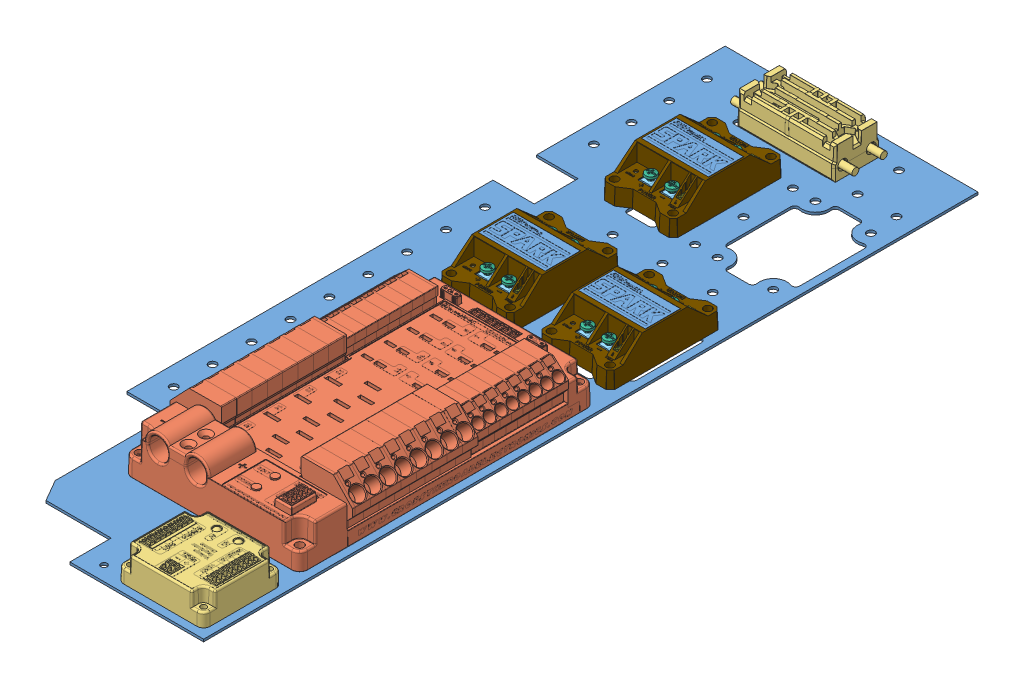
SolidWorks assembly 0001 - 05 - 1010 ELECTRONICS BOARD BOTTOM, configuration Default. Lengths in mm.
Overall size (945.82 43.74 799.08).
117 component instances, 23 part files, 23 mates.
Components (placement in the parent):
- 0001 - 05 - 0001 Reference Geometry-1: 0001 - 05 - 0001 Reference Geometry [Default] at origin size (945.82 0 799.08)
- 0001 - 05 - 1011 Bottom Board-1: 0001 - 05 - 1011 Bottom Board [Default] at origin size (165.1 1.59 505.59)
- PDP_asmb-2: PDP_asmb [Default] at (-272.032 8.2677 231.0895) x (0 0 -1) z (1 0 0) size (192.68 36.15 120.93)
- VRM-3: VRM [Default] at (-242.2924 8.7189 366.7652) size (56.39 19.92 51.56)
- REV_SPARK-1: REV_SPARK [Default] at (-290.8098 -27.4428 120.6986) x (0 0 -1) z (1 0 0) size (73.01 22.15 47.86)
  - RR-SPARK-BD-B-Assembly-1: RR-SPARK-BD-B-Assembly [Default] at (2.3249 6.4587 12.2534) size (55.12 17.9 42.42)
    - RR-SPARK-BD-B-1: RR-SPARK-BD-B [Default] at (27.8945 25.8332 38.0904) size (53.34 3.8 40.64)
    - ScrewTerminalAssembly-1: ScrewTerminalAssembly [Default] at (15.7541 22.7195 39.4261) x (0 0 1) z (-1 0 0) size (7.87 11.69 7.87)
      - ScrewTerminalBase-1: ScrewTerminalBase [Default] at (3.4868 6.6312 8.3972) size (7.87 7.68 7.87)
      - ScrewTerminalScrew-1: ScrewTerminalScrew [Default] at (3.5041 -1.1314 8.5263) x (0.998152 0 -0.060771) z (0.060771 0 0.998152) size (7.16 8.3 7.16)
    - ScrewTerminalAssembly-2: ScrewTerminalAssembly [Default] at (56.3941 22.7195 39.4261) x (0 0 1) z (-1 0 0) size (7.87 11.69 7.87)
      - ScrewTerminalBase-1: ScrewTerminalBase [Default] at (3.4868 6.6312 8.3972) size (7.87 7.68 7.87)
      - ScrewTerminalScrew-1: ScrewTerminalScrew [Default] at (3.5041 -1.1314 8.5263) x (0.998152 0 -0.060771) z (0.060771 0 0.998152) size (7.16 8.3 7.16)
    - ScrewTerminalAssembly-3: ScrewTerminalAssembly [Default] at (15.7541 22.7195 25.4561) x (0 0 1) z (-1 0 0) size (7.87 11.69 7.87)
      - ScrewTerminalBase-1: ScrewTerminalBase [Default] at (3.4868 6.6312 8.3972) size (7.87 7.68 7.87)
      - ScrewTerminalScrew-1: ScrewTerminalScrew [Default] at (3.5041 -1.1314 8.5263) x (0.998152 0 -0.060771) z (0.060771 0 0.998152) size (7.16 8.3 7.16)
    - ScrewTerminalAssembly-4: ScrewTerminalAssembly [Default] at (56.3941 22.7195 25.4561) x (0 0 1) z (-1 0 0) size (7.87 11.69 7.87)
      - ScrewTerminalBase-1: ScrewTerminalBase [Default] at (3.4868 6.6312 8.3972) size (7.87 7.68 7.87)
      - ScrewTerminalScrew-1: ScrewTerminalScrew [Default] at (3.5041 -1.1314 8.5263) x (0.998152 0 -0.060771) z (0.060771 0 0.998152) size (7.16 8.3 7.16)
    - Header-Female-1x3-PPTC031LFBN-RC-1: Header-Female-1x3-PPTC031LFBN-RC [Default] at (7.5745 27.4332 53.3304) size (8.13 11.71 2.54)
    - Header-Female-1x3-PPTC031LFBN-RC-2: Header-Female-1x3-PPTC031LFBN-RC [Default] at (48.2145 27.4332 53.3304) size (8.13 11.71 2.54)
    - Header-Female-1x3-PPTC031LFBN-RC-3: Header-Female-1x3-PPTC031LFBN-RC [Default] at (48.2145 27.4332 55.8704) size (8.13 11.71 2.54)
    - LED-RGB-ThroughHole-1: LED-RGB-ThroughHole [Default] at (48.2145 27.4332 21.5804) x (-1 0 0) z (0 0 -1) size (5.45 12.2 5.9)
    - MOSFET-PSMN1R0-30YLC115-1: MOSFET-PSMN1R0-30YLC115 [Default] at (35.6415 27.4332 27.2954) x (0 0 -1) z (1 0 0) size (5 1.2 6.72)
    - MOSFET-PSMN1R0-30YLC115-2: MOSFET-PSMN1R0-30YLC115 [Default] at (36.5305 27.4332 33.6454) size (5 1.2 6.72)
    - MOSFET-PSMN1R0-30YLC115-3: MOSFET-PSMN1R0-30YLC115 [Default] at (36.5305 27.4332 42.5354) x (-1 0 0) z (0 0 -1) size (5 1.2 6.72)
    - MOSFET-PSMN1R0-30YLC115-4: MOSFET-PSMN1R0-30YLC115 [Default] at (35.6415 27.4332 48.8854) x (0 0 -1) z (1 0 0) size (5 1.2 6.72)
    - Varistor-1: Varistor [Default] at (52.6595 27.4332 22.5964) x (0 0 1) z (-1 0 0) size (3.4 1.02 1.45)
    - Varistor-2: Varistor [Default] at (41.2295 27.4332 53.7114) x (0 0 1) z (-1 0 0) size (3.4 1.02 1.45)
    - Crystal-1: Crystal [Default] at (17.9885 27.4332 48.3774) x (0 0 1) z (-1 0 0) size (5.2 1.5 3.4)
    - Button-PTS645SM43SMTR92LFS-1: Button-PTS645SM43SMTR92LFS [Default] at (8.0825 27.4332 21.5804) size (9 4.3 6)
    - OptoIsolator-TLP118-1: OptoIsolator-TLP118 [Default] at (14.1785 27.4332 50.4094) x (0 0 -1) z (1 0 0) size (7.02 2.2 3.7)
    - GateDriver-A4940KLPTR-T-1: GateDriver-A4940KLPTR-T [Default] at (30.1805 25.8332 53.9654) x (0 0 -1) z (-1 0 0) size (7.8 1.2 6.43)
    - MCU-PIC16F1828-I-GZ-1: MCU-PIC16F1828-I-GZ [Default] at (19.0045 25.8332 52.8224) x (-1 0 0) z (0 0 1) size (4 0.55 4)
    - Capacitor-UCL1V471MNL1GS-1: Capacitor-UCL1V471MNL1GS [Default] at (25.8625 27.4332 46.5994) x (0 0 1) z (-1 0 0) size (10.5 14.3 11.5)
    - Capacitor-UCL1V471MNL1GS-2: Capacitor-UCL1V471MNL1GS [Default] at (25.8625 27.4332 25.2634) x (0 0 1) z (-1 0 0) size (10.5 14.3 11.5)
    - Capacitor-UCL1V471MNL1GS-3: Capacitor-UCL1V471MNL1GS [Default] at (25.8625 27.4332 35.9314) x (0 0 -1) z (1 0 0) size (10.5 14.3 11.5)
    - 1mmborder-1: 1mmborder [Default] at (27.8945 25.8332 38.0904) size (55.12 1.6 42.42)
  - Spark_P01-REV-41_TOPSHELL-1: Spark_P01-REV-41_TOPSHELL [Default] at (30.1178 29.0303 87.4264) x (1 0 0) z (0 1 0) size (73.01 47.86 22.14)
  - heatsink-1: heatsink [Default] at (29.9048 43.475 28.4732) size (25.78 15.4 43.69)
  - Spark_P01-REV-41_bottom_cover-1: Spark_P01-REV-41_bottom_cover [Default] at (30.1178 29.0303 87.4264) x (1 0 0) z (0 -1 0) size (65.7 43.71 2.65)
- REV_SPARK-2: REV_SPARK [Default] at (-356.1591 -27.4428 120.6986) x (0 0 -1) z (1 0 0) size (73.01 22.15 47.86)
  - RR-SPARK-BD-B-Assembly-1: RR-SPARK-BD-B-Assembly [Default] at (2.3249 6.4587 12.2534) size (55.12 17.9 42.42)
    - RR-SPARK-BD-B-1: RR-SPARK-BD-B [Default] at (27.8945 25.8332 38.0904) size (53.34 3.8 40.64)
    - ScrewTerminalAssembly-1: ScrewTerminalAssembly [Default] at (15.7541 22.7195 39.4261) x (0 0 1) z (-1 0 0) size (7.87 11.69 7.87)
      - ScrewTerminalBase-1: ScrewTerminalBase [Default] at (3.4868 6.6312 8.3972) size (7.87 7.68 7.87)
      - ScrewTerminalScrew-1: ScrewTerminalScrew [Default] at (3.5041 -1.1314 8.5263) x (0.998152 0 -0.060771) z (0.060771 0 0.998152) size (7.16 8.3 7.16)
    - ScrewTerminalAssembly-2: ScrewTerminalAssembly [Default] at (56.3941 22.7195 39.4261) x (0 0 1) z (-1 0 0) size (7.87 11.69 7.87)
      - ScrewTerminalBase-1: ScrewTerminalBase [Default] at (3.4868 6.6312 8.3972) size (7.87 7.68 7.87)
      - ScrewTerminalScrew-1: ScrewTerminalScrew [Default] at (3.5041 -1.1314 8.5263) x (0.998152 0 -0.060771) z (0.060771 0 0.998152) size (7.16 8.3 7.16)
    - ScrewTerminalAssembly-3: ScrewTerminalAssembly [Default] at (15.7541 22.7195 25.4561) x (0 0 1) z (-1 0 0) size (7.87 11.69 7.87)
      - ScrewTerminalBase-1: ScrewTerminalBase [Default] at (3.4868 6.6312 8.3972) size (7.87 7.68 7.87)
      - ScrewTerminalScrew-1: ScrewTerminalScrew [Default] at (3.5041 -1.1314 8.5263) x (0.998152 0 -0.060771) z (0.060771 0 0.998152) size (7.16 8.3 7.16)
    - ScrewTerminalAssembly-4: ScrewTerminalAssembly [Default] at (56.3941 22.7195 25.4561) x (0 0 1) z (-1 0 0) size (7.87 11.69 7.87)
      - ScrewTerminalBase-1: ScrewTerminalBase [Default] at (3.4868 6.6312 8.3972) size (7.87 7.68 7.87)
      - ScrewTerminalScrew-1: ScrewTerminalScrew [Default] at (3.5041 -1.1314 8.5263) x (0.998152 0 -0.060771) z (0.060771 0 0.998152) size (7.16 8.3 7.16)
    - Header-Female-1x3-PPTC031LFBN-RC-1: Header-Female-1x3-PPTC031LFBN-RC [Default] at (7.5745 27.4332 53.3304) size (8.13 11.71 2.54)
    - Header-Female-1x3-PPTC031LFBN-RC-2: Header-Female-1x3-PPTC031LFBN-RC [Default] at (48.2145 27.4332 53.3304) size (8.13 11.71 2.54)
    - Header-Female-1x3-PPTC031LFBN-RC-3: Header-Female-1x3-PPTC031LFBN-RC [Default] at (48.2145 27.4332 55.8704) size (8.13 11.71 2.54)
    - LED-RGB-ThroughHole-1: LED-RGB-ThroughHole [Default] at (48.2145 27.4332 21.5804) x (-1 0 0) z (0 0 -1) size (5.45 12.2 5.9)
    - MOSFET-PSMN1R0-30YLC115-1: MOSFET-PSMN1R0-30YLC115 [Default] at (35.6415 27.4332 27.2954) x (0 0 -1) z (1 0 0) size (5 1.2 6.72)
    - MOSFET-PSMN1R0-30YLC115-2: MOSFET-PSMN1R0-30YLC115 [Default] at (36.5305 27.4332 33.6454) size (5 1.2 6.72)
    - MOSFET-PSMN1R0-30YLC115-3: MOSFET-PSMN1R0-30YLC115 [Default] at (36.5305 27.4332 42.5354) x (-1 0 0) z (0 0 -1) size (5 1.2 6.72)
    - MOSFET-PSMN1R0-30YLC115-4: MOSFET-PSMN1R0-30YLC115 [Default] at (35.6415 27.4332 48.8854) x (0 0 -1) z (1 0 0) size (5 1.2 6.72)
    - Varistor-1: Varistor [Default] at (52.6595 27.4332 22.5964) x (0 0 1) z (-1 0 0) size (3.4 1.02 1.45)
    - Varistor-2: Varistor [Default] at (41.2295 27.4332 53.7114) x (0 0 1) z (-1 0 0) size (3.4 1.02 1.45)
    - Crystal-1: Crystal [Default] at (17.9885 27.4332 48.3774) x (0 0 1) z (-1 0 0) size (5.2 1.5 3.4)
    - Button-PTS645SM43SMTR92LFS-1: Button-PTS645SM43SMTR92LFS [Default] at (8.0825 27.4332 21.5804) size (9 4.3 6)
    - OptoIsolator-TLP118-1: OptoIsolator-TLP118 [Default] at (14.1785 27.4332 50.4094) x (0 0 -1) z (1 0 0) size (7.02 2.2 3.7)
    - GateDriver-A4940KLPTR-T-1: GateDriver-A4940KLPTR-T [Default] at (30.1805 25.8332 53.9654) x (0 0 -1) z (-1 0 0) size (7.8 1.2 6.43)
    - MCU-PIC16F1828-I-GZ-1: MCU-PIC16F1828-I-GZ [Default] at (19.0045 25.8332 52.8224) x (-1 0 0) z (0 0 1) size (4 0.55 4)
    - Capacitor-UCL1V471MNL1GS-1: Capacitor-UCL1V471MNL1GS [Default] at (25.8625 27.4332 46.5994) x (0 0 1) z (-1 0 0) size (10.5 14.3 11.5)
    - Capacitor-UCL1V471MNL1GS-2: Capacitor-UCL1V471MNL1GS [Default] at (25.8625 27.4332 25.2634) x (0 0 1) z (-1 0 0) size (10.5 14.3 11.5)
    - Capacitor-UCL1V471MNL1GS-3: Capacitor-UCL1V471MNL1GS [Default] at (25.8625 27.4332 35.9314) x (0 0 -1) z (1 0 0) size (10.5 14.3 11.5)
    - 1mmborder-1: 1mmborder [Default] at (27.8945 25.8332 38.0904) size (55.12 1.6 42.42)
  - Spark_P01-REV-41_TOPSHELL-1: Spark_P01-REV-41_TOPSHELL [Default] at (30.1178 29.0303 87.4264) x (1 0 0) z (0 1 0) size (73.01 47.86 22.14)
  - heatsink-1: heatsink [Default] at (29.9048 43.475 28.4732) size (25.78 15.4 43.69)
  - Spark_P01-REV-41_bottom_cover-1: Spark_P01-REV-41_bottom_cover [Default] at (30.1178 29.0303 87.4264) x (1 0 0) z (0 -1 0) size (65.7 43.71 2.65)
- REV_SPARK-4: REV_SPARK [Default] at (-356.1591 -27.4428 14.1852) x (0 0 -1) z (1 0 0) size (73.01 22.15 47.86)
  - RR-SPARK-BD-B-Assembly-1: RR-SPARK-BD-B-Assembly [Default] at (2.3249 6.4587 12.2534) size (55.12 17.9 42.42)
    - RR-SPARK-BD-B-1: RR-SPARK-BD-B [Default] at (27.8945 25.8332 38.0904) size (53.34 3.8 40.64)
    - ScrewTerminalAssembly-1: ScrewTerminalAssembly [Default] at (15.7541 22.7195 39.4261) x (0 0 1) z (-1 0 0) size (7.87 11.69 7.87)
      - ScrewTerminalBase-1: ScrewTerminalBase [Default] at (3.4868 6.6312 8.3972) size (7.87 7.68 7.87)
      - ScrewTerminalScrew-1: ScrewTerminalScrew [Default] at (3.5041 -1.1314 8.5263) x (0.998152 0 -0.060771) z (0.060771 0 0.998152) size (7.16 8.3 7.16)
    - ScrewTerminalAssembly-2: ScrewTerminalAssembly [Default] at (56.3941 22.7195 39.4261) x (0 0 1) z (-1 0 0) size (7.87 11.69 7.87)
      - ScrewTerminalBase-1: ScrewTerminalBase [Default] at (3.4868 6.6312 8.3972) size (7.87 7.68 7.87)
      - ScrewTerminalScrew-1: ScrewTerminalScrew [Default] at (3.5041 -1.1314 8.5263) x (0.998152 0 -0.060771) z (0.060771 0 0.998152) size (7.16 8.3 7.16)
    - ScrewTerminalAssembly-3: ScrewTerminalAssembly [Default] at (15.7541 22.7195 25.4561) x (0 0 1) z (-1 0 0) size (7.87 11.69 7.87)
      - ScrewTerminalBase-1: ScrewTerminalBase [Default] at (3.4868 6.6312 8.3972) size (7.87 7.68 7.87)
      - ScrewTerminalScrew-1: ScrewTerminalScrew [Default] at (3.5041 -1.1314 8.5263) x (0.998152 0 -0.060771) z (0.060771 0 0.998152) size (7.16 8.3 7.16)
    - ScrewTerminalAssembly-4: ScrewTerminalAssembly [Default] at (56.3941 22.7195 25.4561) x (0 0 1) z (-1 0 0) size (7.87 11.69 7.87)
      - ScrewTerminalBase-1: ScrewTerminalBase [Default] at (3.4868 6.6312 8.3972) size (7.87 7.68 7.87)
      - ScrewTerminalScrew-1: ScrewTerminalScrew [Default] at (3.5041 -1.1314 8.5263) x (0.998152 0 -0.060771) z (0.060771 0 0.998152) size (7.16 8.3 7.16)
    - Header-Female-1x3-PPTC031LFBN-RC-1: Header-Female-1x3-PPTC031LFBN-RC [Default] at (7.5745 27.4332 53.3304) size (8.13 11.71 2.54)
    - Header-Female-1x3-PPTC031LFBN-RC-2: Header-Female-1x3-PPTC031LFBN-RC [Default] at (48.2145 27.4332 53.3304) size (8.13 11.71 2.54)
    - Header-Female-1x3-PPTC031LFBN-RC-3: Header-Female-1x3-PPTC031LFBN-RC [Default] at (48.2145 27.4332 55.8704) size (8.13 11.71 2.54)
    - LED-RGB-ThroughHole-1: LED-RGB-ThroughHole [Default] at (48.2145 27.4332 21.5804) x (-1 0 0) z (0 0 -1) size (5.45 12.2 5.9)
    - MOSFET-PSMN1R0-30YLC115-1: MOSFET-PSMN1R0-30YLC115 [Default] at (35.6415 27.4332 27.2954) x (0 0 -1) z (1 0 0) size (5 1.2 6.72)
    - MOSFET-PSMN1R0-30YLC115-2: MOSFET-PSMN1R0-30YLC115 [Default] at (36.5305 27.4332 33.6454) size (5 1.2 6.72)
    - MOSFET-PSMN1R0-30YLC115-3: MOSFET-PSMN1R0-30YLC115 [Default] at (36.5305 27.4332 42.5354) x (-1 0 0) z (0 0 -1) size (5 1.2 6.72)
    - MOSFET-PSMN1R0-30YLC115-4: MOSFET-PSMN1R0-30YLC115 [Default] at (35.6415 27.4332 48.8854) x (0 0 -1) z (1 0 0) size (5 1.2 6.72)
    - Varistor-1: Varistor [Default] at (52.6595 27.4332 22.5964) x (0 0 1) z (-1 0 0) size (3.4 1.02 1.45)
    - Varistor-2: Varistor [Default] at (41.2295 27.4332 53.7114) x (0 0 1) z (-1 0 0) size (3.4 1.02 1.45)
    - Crystal-1: Crystal [Default] at (17.9885 27.4332 48.3774) x (0 0 1) z (-1 0 0) size (5.2 1.5 3.4)
    - Button-PTS645SM43SMTR92LFS-1: Button-PTS645SM43SMTR92LFS [Default] at (8.0825 27.4332 21.5804) size (9 4.3 6)
    - OptoIsolator-TLP118-1: OptoIsolator-TLP118 [Default] at (14.1785 27.4332 50.4094) x (0 0 -1) z (1 0 0) size (7.02 2.2 3.7)
    - GateDriver-A4940KLPTR-T-1: GateDriver-A4940KLPTR-T [Default] at (30.1805 25.8332 53.9654) x (0 0 -1) z (-1 0 0) size (7.8 1.2 6.43)
    - MCU-PIC16F1828-I-GZ-1: MCU-PIC16F1828-I-GZ [Default] at (19.0045 25.8332 52.8224) x (-1 0 0) z (0 0 1) size (4 0.55 4)
    - Capacitor-UCL1V471MNL1GS-1: Capacitor-UCL1V471MNL1GS [Default] at (25.8625 27.4332 46.5994) x (0 0 1) z (-1 0 0) size (10.5 14.3 11.5)
    - Capacitor-UCL1V471MNL1GS-2: Capacitor-UCL1V471MNL1GS [Default] at (25.8625 27.4332 25.2634) x (0 0 1) z (-1 0 0) size (10.5 14.3 11.5)
    - Capacitor-UCL1V471MNL1GS-3: Capacitor-UCL1V471MNL1GS [Default] at (25.8625 27.4332 35.9314) x (0 0 -1) z (1 0 0) size (10.5 14.3 11.5)
    - 1mmborder-1: 1mmborder [Default] at (27.8945 25.8332 38.0904) size (55.12 1.6 42.42)
  - Spark_P01-REV-41_TOPSHELL-1: Spark_P01-REV-41_TOPSHELL [Default] at (30.1178 29.0303 87.4264) x (1 0 0) z (0 1 0) size (73.01 47.86 22.14)
  - heatsink-1: heatsink [Default] at (29.9048 43.475 28.4732) size (25.78 15.4 43.69)
  - Spark_P01-REV-41_bottom_cover-1: Spark_P01-REV-41_bottom_cover [Default] at (30.1178 29.0303 87.4264) x (1 0 0) z (0 -1 0) size (65.7 43.71 2.65)
- Victor SP-1: Victor SP [Default] at (-293.3197 7.7573 -79.0575) x (0 0 -1) z (1 0 0) size (30.24 20.93 80)
- Circuit Breaker 120A-1: Circuit Breaker 120A [Default] at (-238.125 6.4135 -14.097) x (0 0 -1) z (1 0 0) size (73.72 42.2 48.95)
Mates (geometry in assembly coordinates):
- Coincident1: coordinate: point of ?
- Coincident2: coordinate: point of 0001 - 05 - 0001 Reference Geometry-1; point of 0001 - 05 - 1011 Bottom Board-1
- Concentric6: concentric anti-aligned: cylinder of 0001 - 05 - 1011 Bottom Board-1 through (-219.835 0 326.5427) axis (0 1 0) radius 2.667; cylinder of PDP_asmb-2 through (-219.835 10.5537 326.5427) axis (0 -1 0) radius 2.667
- Coincident7: coincident anti-aligned: plane of 0001 - 05 - 1011 Bottom Board-1 through (0 1.5875 0) normal (0 1 0); plane of PDP_asmb-2 through (-214.628 1.5875 139.0653) normal (0 -1 0)
- Parallel6: parallel aligned: line of 0001 - 05 - 1011 Bottom Board-1 through (-237.4335 1.5875 136.652) axis (-1 0 0); line of PDP_asmb-2 through (-219.8387 1.8459 139.0698) axis (-1 0 0)
- Coincident11: coincident anti-aligned: plane of 0001 - 05 - 1011 Bottom Board-1 through (0 1.5875 0) normal (0 1 0); plane of VRM-3 through (-218.948 1.5875 347.218) normal (0 -1 0)
- Concentric10: concentric anti-aligned: cylinder of 0001 - 05 - 1011 Bottom Board-1 through (-218.948 0 390.144) axis (0 1 0) radius 1.905; cylinder of VRM-3 through (-218.948 19.6249 390.144) axis (0 -1 0) radius 1.905
- Concentric11: concentric anti-aligned: cylinder of 0001 - 05 - 1011 Bottom Board-1 through (-221.2382 0 122.4895) axis (0 1 0) radius 2.5527; cylinder of REV_SPARK-1/Spark_P01-REV-41_TOPSHELL-1 through (-221.2382 12.245 122.4895) axis (0 -1 0) radius 2.5527
- Coincident13: coincident anti-aligned: plane of 0001 - 05 - 1011 Bottom Board-1 through (0 1.5875 0) normal (0 1 0); plane of REV_SPARK-1/Spark_P01-REV-41_TOPSHELL-1 through (-240.4814 1.5875 90.6119) normal (0 -1 0)
- Parallel10: parallel aligned: line of 0001 - 05 - 1011 Bottom Board-1 through (-232.4449 1.5875 53.848) axis (-1 0 0); line of REV_SPARK-1/Spark_P01-REV-41_TOPSHELL-1 through (-233.0919 1.5875 58.672) axis (-1 0 0)
- Concentric13: concentric anti-aligned: cylinder of 0001 - 05 - 1011 Bottom Board-1 through (-286.5874 0 122.4895) axis (0 1 0) radius 2.5527; cylinder of REV_SPARK-2/Spark_P01-REV-41_TOPSHELL-1 through (-286.5874 12.245 122.4895) axis (0 -1 0) radius 2.5527
- Coincident17: coincident anti-aligned: plane of 0001 - 05 - 1011 Bottom Board-1 through (0 1.5875 0) normal (0 1 0); plane of REV_SPARK-2/Spark_P01-REV-41_TOPSHELL-1 through (-305.8306 1.5875 90.6119) normal (0 -1 0)
- Parallel12: parallel: line of 0001 - 05 - 1011 Bottom Board-1 through (-297.7942 1.5875 53.848) axis (-1 0 0); plane of REV_SPARK-2/Spark_P01-REV-41_TOPSHELL-1 through (-313.1124 1.5875 58.672) normal (0 0.043619 -0.999048)
- Concentric17: concentric anti-aligned: cylinder of 0001 - 05 - 1011 Bottom Board-1 through (-286.5874 0 15.9762) axis (0 1 0) radius 2.5527; cylinder of REV_SPARK-4/Spark_P01-REV-41_TOPSHELL-1 through (-286.5874 12.245 15.9762) axis (0 -1 0) radius 2.5527
- Coincident20: coincident anti-aligned: plane of 0001 - 05 - 1011 Bottom Board-1 through (0 1.5875 0) normal (0 1 0); plane of REV_SPARK-4/Spark_P01-REV-41_TOPSHELL-1 through (-305.8306 1.5875 -15.9014) normal (0 -1 0)
- Parallel14: parallel: line of 0001 - 05 - 1011 Bottom Board-1 through (-297.9007 1.5875 -52.07) axis (-1 0 0); plane of REV_SPARK-4/Spark_P01-REV-41_TOPSHELL-1 through (-313.1124 1.5875 -47.8413) normal (0 0.043619 -0.999048)
- Concentric18: concentric aligned: cylinder of 0001 - 05 - 1011 Bottom Board-1 through (-267.9197 0 -79.0575) axis (0 1 0) radius 1.0922; cone of Victor SP-1 through (-267.9197 9.2075 -79.0575) axis (0 1 0)
- Coincident21: coincident anti-aligned: plane of 0001 - 05 - 1011 Bottom Board-1 through (0 1.5875 0) normal (0 1 0); plane of Victor SP-1 through (-261.5697 1.5875 -94.1905) normal (0 -1 0)
- Parallel17: parallel: line of 0001 - 05 - 1011 Bottom Board-1 through (-267.716 1.5875 -93.345) axis (-1 0 0); plane of Victor SP-1 through (-261.5697 9.2075 -94.0575) normal (0 0.017452 -0.999848)
- Concentric19: concentric anti-aligned: cylinder of 0001 - 05 - 1011 Bottom Board-1 through (-266.7 0 390.144) axis (0 1 0) radius 1.905; cylinder of VRM-3 through (-266.7 19.6249 390.144) axis (0 -1 0) radius 1.905
- Concentric20: concentric anti-aligned: cylinder of 0001 - 05 - 1011 Bottom Board-1 through (-224.155 0 14.478) axis (0 1 0) radius 3.175; cylinder of Circuit Breaker 120A-1 through (-224.155 11.4935 14.478) axis (0 -1 0) radius 3.429
- Parallel18: parallel aligned: line of 0001 - 05 - 1011 Bottom Board-1 through (-217.17 1.5875 -46.482) axis (-1 0 0); line of Circuit Breaker 120A-1 through (-217.043 1.5875 -50.927) axis (-1 0 0)
- Coincident23: coincident anti-aligned: plane of 0001 - 05 - 1011 Bottom Board-1 through (0 1.5875 0) normal (0 1 0); plane of Circuit Breaker 120A-1 through (-220.6395 1.5875 -45.5839) normal (0 -1 0)
